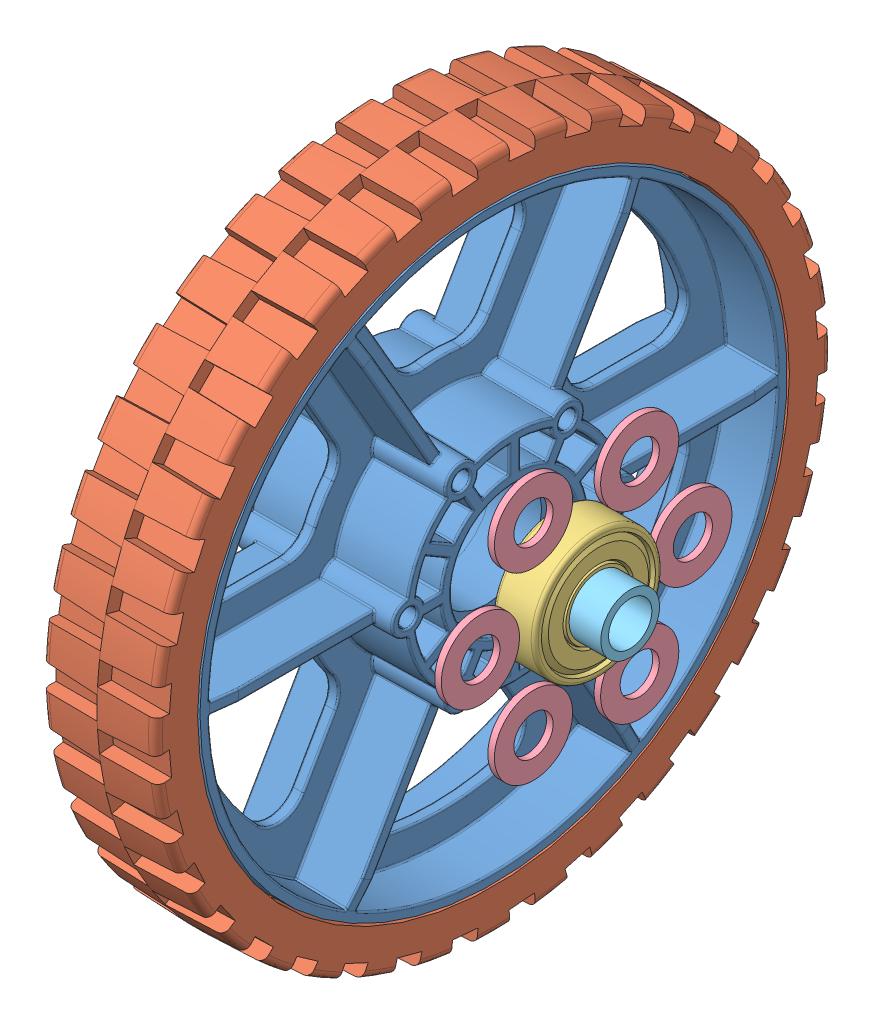
SolidWorks assembly 6 HiGrip with bearings, pulleys and spacers, configuration Default. Lengths in mm.
Overall size (85.56 152.4 152.4).
13 component instances, 6 part files, 0 mates.
Components (placement in the parent):
- 6 HiGrip Wheel Assembly Rev II-1: 6 HiGrip Wheel Assembly Rev II [Default] at (83.7987 67.439 110.9939) size (34.93 152.4 152.4)
  - 6 wheel Rev 4-1: 6 wheel Rev 4 [Default] at (-52.6446 9.4231 21.378) size (34.93 132.08 132.08)
  - 6 wheel tread II-1: 6 wheel tread II [Default] at (-65.3446 9.4231 21.378) x (0 0 -1) z (1 0 0) size (152.4 152.4 25.58)
- Bearing_1614ZZ-1: Bearing_1614ZZ [Default] at (62.612 76.862 132.3719) x (0 -0.157148 -0.987575) z (-1 0 0) size (28.58 28.58 9.53)
- Bearing_1614ZZ-2: Bearing_1614ZZ [Default] at (15.2791 76.862 132.3719) x (0 0 -1) z (1 0 0) size (28.58 28.58 9.53)
- Washer_5-16-1: Washer_5-16 [Default] at (63.247 76.8605 108.5602) x (0 0.946124 0.323805) z (1 0 0) size (17.53 17.53 1.47)
- Washer_5-16-2: Washer_5-16 [Default] at (63.247 97.4833 120.4656) x (0 0.770474 -0.637472) z (1 0 0) size (17.53 17.53 1.47)
- Washer_5-16-3: Washer_5-16 [Default] at (63.247 56.2398 144.2799) x (0 0 -1) z (1 0 0) size (17.53 17.53 1.47)
- Washer_5-16-4: Washer_5-16 [Default] at (63.247 76.8625 156.1852) x (0 -0.95788 -0.287168) z (1 0 0) size (17.53 17.53 1.47)
- Washer_5-16-5: Washer_5-16 [Default] at (63.247 97.4843 144.2781) x (0 -0.653102 0.75727) z (1 0 0) size (17.53 17.53 1.47)
- Washer_5-16-6: Washer_5-16 [Default] at (63.247 56.2388 120.4674) x (0 -0.977348 -0.211637) z (1 0 0) size (17.53 17.53 1.47)
- Spacer_0.28x0.382-1: Spacer_0.28x0.382 [Default] at (74.4865 76.862 132.3719) x (0 -0.35357 0.935408) z (-1 0 0) size (13.16 13.16 7.11)
- Spacer_0.85x0.38-1: Spacer_0.85x0.38 [Default] at (-11.0734 76.862 132.3719) x (0 0 -1) z (1 0 0) size (19.05 19.05 21.59)
